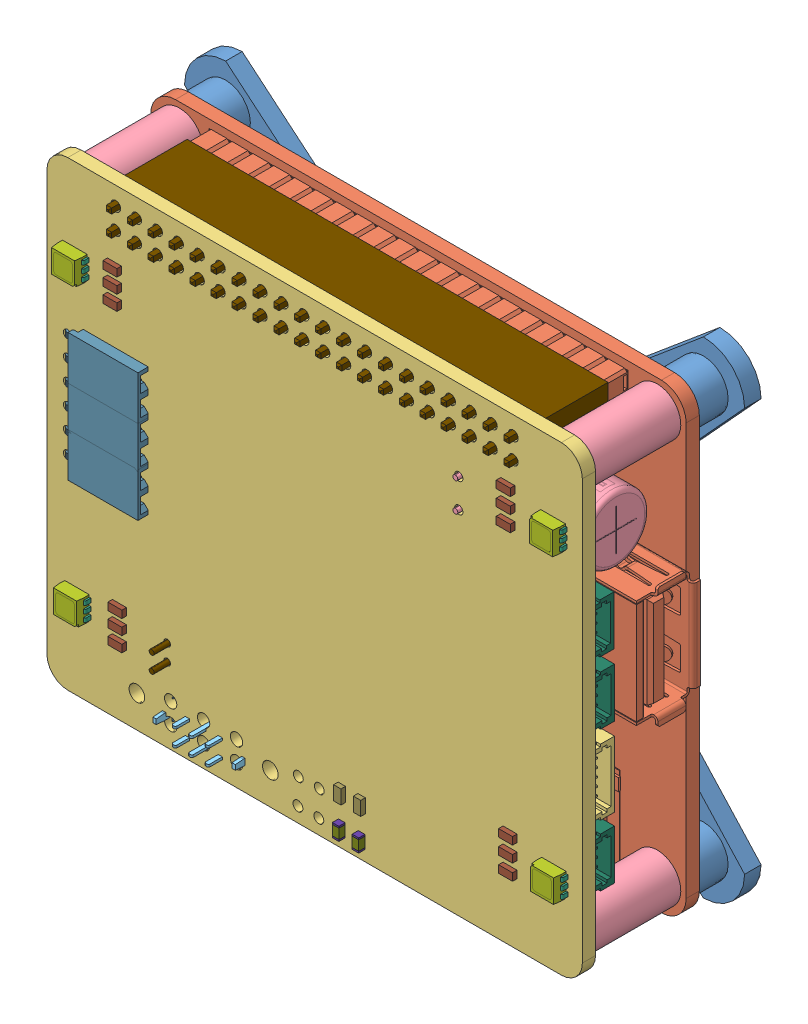
SolidWorks assembly ulemine elektroonika.pi3+, configuration Default. Lengths in mm.
Overall size (68.25 60 22.11).
305 component instances, 41 part files, 9 mates.
Components (placement in the parent):
- Raspberry kinnitus v1.1-1: Raspberry kinnitus v1.1 [Default] at (14.7608 -17.7793 -6.33) x (0 1 0) z (1 0 0) size (59 6 68)
- STMf303 hat + RPi 3A+-1: STMf303 hat + RPi 3A+ [Default] at (-28.0333 0.157 -11.5935) size (68.17 58.5 17.95)
  - Raspberry PI 3 Model A+-1: Raspberry PI 3 Model A+ [Défaut] at (135.3946 10.6154 11.2635) size (68.17 58.5 11.94)
  - FC_PiHat_REV1-1: FC_PiHat_REV1 [Default] at (41.2941 -16.4646 23.8635) x (-1 0 0) z (0 0 -1) size (65 56 12.01)
    - FC_PiHat_REV1.step-1: FC_PiHat_REV1.step [Default] at origin size (65 56 12.01)
      - J7FC_PiHat_REV1.step-1: J7FC_PiHat_REV1.step [Default] at origin size (8 4.95 2.96)
        - SM06B-SRSS-TB.step-1: SM06B-SRSS-TB.step [Default] at (13.3 4.6 -0.3) x (1 0 0) z (0 -1 0) size (8 2.96 4.95)
      - C10FC_PiHat_REV1.step-1: C10FC_PiHat_REV1.step [Default] at origin size (13.96 8.06 10.04)
        - User_Library-Cap_electro_8x11_5x3_5mm_RA.step-1: User_Library-Cap_electro_8x11_5x3_5mm_RA.step [Default] at (13.5254 44.5 4) x (0 1 0) z (0 0 1) size (8.06 13.96 10.04)
      - J11FC_PiHat_REV1.step-1: J11FC_PiHat_REV1.step [Default] at origin size (10 6 9.8)
        - User_Library-EG1940-ND.step-1: User_Library-EG1940-ND.step [Default] at (40.9499 0.2249 0) x (1 0 0) z (0 0 1) size (10 6 9.8)
      - D4FC_PiHat_REV1.step-1: D4FC_PiHat_REV1.step [Default] at origin size (3.4 2.8 1.85)
        - User_Library-RGB_LED_Zwart_ASMT-YTC2-0AA02.step-1: User_Library-RGB_LED_Zwart_ASMT-YTC2-0AA02.step [Default] at (2.2908 8.9737 -1.6023) x (-1 0 0) z (0 -1 0) size (3.4 1.85 2.8)
          - Pootje_RGB_LED.step-1: Pootje_RGB_LED.step [Default] at (-0.3594 -0.1975 0.3238) size (0.9 1.1 0.5)
          - ASMT-YTC2-0AA02.step-1: ASMT-YTC2-0AA02.step [Default] at (-2.6594 -0.3475 0.5738) size (3 1.8 2.8)
          - Pootje_RGB_LED.step-2: Pootje_RGB_LED.step [Default] at (-0.3594 -0.1975 -0.5762) size (0.9 1.1 0.5)
          - Pootje_RGB_LED.step-3: Pootje_RGB_LED.step [Default] at (-0.3594 -0.1975 -1.4762) size (0.9 1.1 0.5)
          - Pootje_RGB_LED.step-4: Pootje_RGB_LED.step [Default] at (-1.9594 -0.1975 -1.9762) x (-1 0 0) z (0 0 -1) size (0.9 1.1 0.5)
          - Pootje_RGB_LED.step-5: Pootje_RGB_LED.step [Default] at (-1.9594 -0.1975 -1.0762) x (-1 0 0) z (0 0 -1) size (0.9 1.1 0.5)
          - Pootje_RGB_LED.step-6: Pootje_RGB_LED.step [Default] at (-1.9594 -0.1975 -0.1762) x (-1 0 0) z (0 0 -1) size (0.9 1.1 0.5)
      - D3FC_PiHat_REV1.step-1: D3FC_PiHat_REV1.step [Default] at origin size (3.4 2.8 1.85)
        - User_Library-RGB_LED_Zwart_ASMT-YTC2-0AA02.step-1: User_Library-RGB_LED_Zwart_ASMT-YTC2-0AA02.step [Default] at (2.3908 45.4737 -1.6023) x (-1 0 0) z (0 -1 0) size (3.4 1.85 2.8)
          - Pootje_RGB_LED.step-1: Pootje_RGB_LED.step [Default] at (-0.3594 -0.1975 0.3238) size (0.9 1.1 0.5)
          - ASMT-YTC2-0AA02.step-1: ASMT-YTC2-0AA02.step [Default] at (-2.6594 -0.3475 0.5738) size (3 1.8 2.8)
          - Pootje_RGB_LED.step-2: Pootje_RGB_LED.step [Default] at (-0.3594 -0.1975 -0.5762) size (0.9 1.1 0.5)
          - Pootje_RGB_LED.step-3: Pootje_RGB_LED.step [Default] at (-0.3594 -0.1975 -1.4762) size (0.9 1.1 0.5)
          - Pootje_RGB_LED.step-4: Pootje_RGB_LED.step [Default] at (-1.9594 -0.1975 -1.9762) x (-1 0 0) z (0 0 -1) size (0.9 1.1 0.5)
          - Pootje_RGB_LED.step-5: Pootje_RGB_LED.step [Default] at (-1.9594 -0.1975 -1.0762) x (-1 0 0) z (0 0 -1) size (0.9 1.1 0.5)
          - Pootje_RGB_LED.step-6: Pootje_RGB_LED.step [Default] at (-1.9594 -0.1975 -0.1762) x (-1 0 0) z (0 0 -1) size (0.9 1.1 0.5)
      - D2FC_PiHat_REV1.step-1: D2FC_PiHat_REV1.step [Default] at origin size (3.4 2.8 1.85)
        - User_Library-RGB_LED_Zwart_ASMT-YTC2-0AA02.step-1: User_Library-RGB_LED_Zwart_ASMT-YTC2-0AA02.step [Default] at (62.5092 10.7763 -1.6023) x (1 0 0) z (0 1 0) size (3.4 1.85 2.8)
          - Pootje_RGB_LED.step-1: Pootje_RGB_LED.step [Default] at (-0.3594 -0.1975 0.3238) size (0.9 1.1 0.5)
          - ASMT-YTC2-0AA02.step-1: ASMT-YTC2-0AA02.step [Default] at (-2.6594 -0.3475 0.5738) size (3 1.8 2.8)
          - Pootje_RGB_LED.step-2: Pootje_RGB_LED.step [Default] at (-0.3594 -0.1975 -0.5762) size (0.9 1.1 0.5)
          - Pootje_RGB_LED.step-3: Pootje_RGB_LED.step [Default] at (-0.3594 -0.1975 -1.4762) size (0.9 1.1 0.5)
          - Pootje_RGB_LED.step-4: Pootje_RGB_LED.step [Default] at (-1.9594 -0.1975 -1.9762) x (-1 0 0) z (0 0 -1) size (0.9 1.1 0.5)
          - Pootje_RGB_LED.step-5: Pootje_RGB_LED.step [Default] at (-1.9594 -0.1975 -1.0762) x (-1 0 0) z (0 0 -1) size (0.9 1.1 0.5)
          - Pootje_RGB_LED.step-6: Pootje_RGB_LED.step [Default] at (-1.9594 -0.1975 -0.1762) x (-1 0 0) z (0 0 -1) size (0.9 1.1 0.5)
      - D1FC_PiHat_REV1.step-1: D1FC_PiHat_REV1.step [Default] at origin size (3.4 2.8 1.85)
        - User_Library-RGB_LED_Zwart_ASMT-YTC2-0AA02.step-1: User_Library-RGB_LED_Zwart_ASMT-YTC2-0AA02.step [Default] at (62.7592 46.4263 -1.6023) x (1 0 0) z (0 1 0) size (3.4 1.85 2.8)
          - Pootje_RGB_LED.step-1: Pootje_RGB_LED.step [Default] at (-0.3594 -0.1975 0.3238) size (0.9 1.1 0.5)
          - ASMT-YTC2-0AA02.step-1: ASMT-YTC2-0AA02.step [Default] at (-2.6594 -0.3475 0.5738) size (3 1.8 2.8)
          - Pootje_RGB_LED.step-2: Pootje_RGB_LED.step [Default] at (-0.3594 -0.1975 -0.5762) size (0.9 1.1 0.5)
          - Pootje_RGB_LED.step-3: Pootje_RGB_LED.step [Default] at (-0.3594 -0.1975 -1.4762) size (0.9 1.1 0.5)
          - Pootje_RGB_LED.step-4: Pootje_RGB_LED.step [Default] at (-1.9594 -0.1975 -1.9762) x (-1 0 0) z (0 0 -1) size (0.9 1.1 0.5)
          - Pootje_RGB_LED.step-5: Pootje_RGB_LED.step [Default] at (-1.9594 -0.1975 -1.0762) x (-1 0 0) z (0 0 -1) size (0.9 1.1 0.5)
          - Pootje_RGB_LED.step-6: Pootje_RGB_LED.step [Default] at (-1.9594 -0.1975 -0.1762) x (-1 0 0) z (0 0 -1) size (0.9 1.1 0.5)
      - S1FC_PiHat_REV1.step-1: S1FC_PiHat_REV1.step [Default] at origin size (4.1 4.1 0.81)
        - 5843174976.step-1: 5843174976.step [Default] at (40.7 32.3 0) size (4.1 4.1 0.81)
          - Body.step-1: Body.step [Default] at (-2.05 -2.05 0)
            - Open_CASCADE_STEP_translator_6.8_14.2.1.x_t-1: Open_CASCADE_STEP_translator_6.8_14.2.1.x_t [Default] at origin
          - Open_CASCADE_STEP_translator_6.8_14.1.step-1: Open_CASCADE_STEP_translator_6.8_14.1.step [Default] at (-2.05 -2.05 0) size (0.52 0.52 0.01)
          - Thermal_Shape.step-1: Thermal_Shape.step [Default] at (-1.3 -1.35 -0.001) size (2.6 2.7 0)
          - Pin_Shape.step-1: Pin_Shape.step [Default] at (-2.05 -1.37 0) size (0.35 0.24 0)
          - Pin_Shape.step-2: Pin_Shape.step [Default] at (2.05 1.37 0) x (-1 0 0) z (0 0 1) size (0.35 0.24 0)
          - Pin_Shape.step-3: Pin_Shape.step [Default] at (-2.05 -0.87 0) size (0.35 0.24 0)
          - Pin_Shape.step-4: Pin_Shape.step [Default] at (2.05 0.87 0) x (-1 0 0) z (0 0 1) size (0.35 0.24 0)
          - Pin_Shape.step-5: Pin_Shape.step [Default] at (-2.05 -0.37 0) size (0.35 0.24 0)
          - Pin_Shape.step-6: Pin_Shape.step [Default] at (2.05 0.37 0) x (-1 0 0) z (0 0 1) size (0.35 0.24 0)
          - Pin_Shape.step-7: Pin_Shape.step [Default] at (-2.05 0.13 0) size (0.35 0.24 0)
          - Pin_Shape.step-8: Pin_Shape.step [Default] at (2.05 -0.13 0) x (-1 0 0) z (0 0 1) size (0.35 0.24 0)
          - Pin_Shape.step-9: Pin_Shape.step [Default] at (-2.05 0.63 0) size (0.35 0.24 0)
          - Pin_Shape.step-10: Pin_Shape.step [Default] at (2.05 -0.63 0) x (-1 0 0) z (0 0 1) size (0.35 0.24 0)
          - Pin_Shape.step-11: Pin_Shape.step [Default] at (-2.05 1.13 0) size (0.35 0.24 0)
          - Pin_Shape.step-12: Pin_Shape.step [Default] at (2.05 -1.13 0) x (-1 0 0) z (0 0 1) size (0.35 0.24 0)
          - Pin_Shape.step-13: Pin_Shape.step [Default] at (-1.13 -2.05 0) x (0 1 0) z (0 0 1) size (0.35 0.24 0)
          - Pin_Shape.step-14: Pin_Shape.step [Default] at (1.13 2.05 0) x (0 -1 0) z (0 0 1) size (0.35 0.24 0)
          - Pin_Shape.step-15: Pin_Shape.step [Default] at (-0.63 -2.05 0) x (0 1 0) z (0 0 1) size (0.35 0.24 0)
          - Pin_Shape.step-16: Pin_Shape.step [Default] at (0.63 2.05 0) x (0 -1 0) z (0 0 1) size (0.35 0.24 0)
          - Pin_Shape.step-17: Pin_Shape.step [Default] at (-0.13 -2.05 0) x (0 1 0) z (0 0 1) size (0.35 0.24 0)
          - Pin_Shape.step-18: Pin_Shape.step [Default] at (0.13 2.05 0) x (0 -1 0) z (0 0 1) size (0.35 0.24 0)
          - Pin_Shape.step-19: Pin_Shape.step [Default] at (0.37 -2.05 0) x (0 1 0) z (0 0 1) size (0.35 0.24 0)
          - Pin_Shape.step-20: Pin_Shape.step [Default] at (-0.37 2.05 0) x (0 -1 0) z (0 0 1) size (0.35 0.24 0)
          - Pin_Shape.step-21: Pin_Shape.step [Default] at (0.87 -2.05 0) x (0 1 0) z (0 0 1) size (0.35 0.24 0)
          - Pin_Shape.step-22: Pin_Shape.step [Default] at (-0.87 2.05 0) x (0 -1 0) z (0 0 1) size (0.35 0.24 0)
          - Pin_Shape.step-23: Pin_Shape.step [Default] at (1.37 -2.05 0) x (0 1 0) z (0 0 1) size (0.35 0.24 0)
          - Pin_Shape.step-24: Pin_Shape.step [Default] at (-1.37 2.05 0) x (0 -1 0) z (0 0 1) size (0.35 0.24 0)
      - R14FC_PiHat_REV1.step-1: R14FC_PiHat_REV1.step [Default] at origin size (1.7 0.9 0.55)
        - 6063442624.step-1: 6063442624.step [Default] at (8.7742 7.9 -2.1523) size (1.7 0.9 0.55)
          - Extruded.step-1: Extruded.step [Default] at origin size (1.7 0.9 0.55)
      - R13FC_PiHat_REV1.step-1: R13FC_PiHat_REV1.step [Default] at origin size (1.7 0.9 0.55)
        - 6063442624.step-1: 6063442624.step [Default] at (8.7742 9.8048 -2.1523) size (1.7 0.9 0.55)
          - Extruded.step-1: Extruded.step [Default] at origin size (1.7 0.9 0.55)
      - R12FC_PiHat_REV1.step-1: R12FC_PiHat_REV1.step [Default] at origin size (1.7 0.9 0.55)
        - 6063442624.step-1: 6063442624.step [Default] at (8.7742 11.7 -2.1523) size (1.7 0.9 0.55)
          - Extruded.step-1: Extruded.step [Default] at origin size (1.7 0.9 0.55)
      - R11FC_PiHat_REV1.step-1: R11FC_PiHat_REV1.step [Default] at origin size (1.7 0.9 0.55)
        - 6063442624.step-1: 6063442624.step [Default] at (9.05 44.4 -2.1523) size (1.7 0.9 0.55)
          - Extruded.step-1: Extruded.step [Default] at origin size (1.7 0.9 0.55)
      - R10FC_PiHat_REV1.step-1: R10FC_PiHat_REV1.step [Default] at origin size (1.7 0.9 0.55)
        - 6063442624.step-1: 6063442624.step [Default] at (9.05 46.3 -2.1523) size (1.7 0.9 0.55)
          - Extruded.step-1: Extruded.step [Default] at origin size (1.7 0.9 0.55)
      - R9FC_PiHat_REV1.step-1: R9FC_PiHat_REV1.step [Default] at origin size (0.9 1.7 0.55)
        - 6063442432.step-1: 6063442432.step [Default] at (59.9 29.7 0) size (0.9 1.7 0.55)
          - Extruded-0.step-1: Extruded-0.step [Default] at origin size (0.9 1.7 0.55)
      - R8FC_PiHat_REV1.step-1: R8FC_PiHat_REV1.step [Default] at origin size (1.7 0.9 0.55)
        - 6063442624.step-1: 6063442624.step [Default] at (9.05 48.2 -2.1523) size (1.7 0.9 0.55)
          - Extruded.step-1: Extruded.step [Default] at origin size (1.7 0.9 0.55)
      - R7FC_PiHat_REV1.step-1: R7FC_PiHat_REV1.step [Default] at origin size (1.84 1.84 0.55)
        - 6063441088.step-1: 6063441088.step [Default] at (39.9 37.9 0) size (1.84 1.84 0.55)
          - Extruded-1.step-1: Extruded-1.step [Default] at origin size (1.84 1.84 0.55)
      - R6FC_PiHat_REV1.step-1: R6FC_PiHat_REV1.step [Default] at origin size (1.7 0.9 0.55)
        - 6063442624.step-1: 6063442624.step [Default] at (56.2 11.8 -2.1523) size (1.7 0.9 0.55)
          - Extruded.step-1: Extruded.step [Default] at origin size (1.7 0.9 0.55)
      - R5FC_PiHat_REV1.step-1: R5FC_PiHat_REV1.step [Default] at origin size (1.7 0.9 0.55)
        - 6063442624.step-1: 6063442624.step [Default] at (56.2 10 -2.1523) size (1.7 0.9 0.55)
          - Extruded.step-1: Extruded.step [Default] at origin size (1.7 0.9 0.55)
      - R4FC_PiHat_REV1.step-1: R4FC_PiHat_REV1.step [Default] at origin size (1.7 0.9 0.55)
        - 6063442624.step-1: 6063442624.step [Default] at (56.2 8.2 -2.1523) size (1.7 0.9 0.55)
          - Extruded.step-1: Extruded.step [Default] at origin size (1.7 0.9 0.55)
      - R3FC_PiHat_REV1.step-1: R3FC_PiHat_REV1.step [Default] at origin size (1.7 0.9 0.55)
        - 6063442624.step-1: 6063442624.step [Default] at (56.8 47.4 -2.1523) size (1.7 0.9 0.55)
          - Extruded.step-1: Extruded.step [Default] at origin size (1.7 0.9 0.55)
      - R2FC_PiHat_REV1.step-1: R2FC_PiHat_REV1.step [Default] at origin size (1.7 0.9 0.55)
        - 6063442624.step-1: 6063442624.step [Default] at (56.8 45.6 -2.1523) size (1.7 0.9 0.55)
          - Extruded.step-1: Extruded.step [Default] at origin size (1.7 0.9 0.55)
      - R1FC_PiHat_REV1.step-1: R1FC_PiHat_REV1.step [Default] at origin size (1.7 0.9 0.55)
        - 6063442624.step-1: 6063442624.step [Default] at (56.8 43.8 -2.1523) size (1.7 0.9 0.55)
          - Extruded.step-1: Extruded.step [Default] at origin size (1.7 0.9 0.55)
      - J8FC_PiHat_REV1.step-1: J8FC_PiHat_REV1.step [Default] at origin size (4.95 8 2.96)
        - SM06B-SRSS-TB.step-1: SM06B-SRSS-TB.step [Default] at (4.55 19.8 -0.3) x (0 -1 0) z (-1 0 0) size (8 2.96 4.95)
      - J6FC_PiHat_REV1.step-1: J6FC_PiHat_REV1.step [Default] at origin size (10.06 15.53 5.7)
        - female_header_a-bl254-ea-g02d.step-1: female_header_a-bl254-ea-g02d.step [Default] at (61.2001 31.0851 -1.6023) x (0 -1 0) z (0 0 -1) size (5.33 10.06 5.7)
        - female_header_a-bl254-ea-g02d.step-2: female_header_a-bl254-ea-g02d.step [Default] at (61.2001 26.0099 -1.6023) x (0 -1 0) z (0 0 -1) size (5.33 10.06 5.7)
        - female_header_a-bl254-ea-g02d.step-3: female_header_a-bl254-ea-g02d.step [Default] at (61.2001 36.2099 -1.6023) x (0 -1 0) z (0 0 -1) size (5.33 10.06 5.7)
      - J4FC_PiHat_REV1.step-1: J4FC_PiHat_REV1.step [Default] at origin size (4.95 6 2.96)
        - SM04B-SRSS-TB.step-1: SM04B-SRSS-TB.step [Default] at (4.55 28.375 -0.3) x (0 -1 0) z (-1 0 0) size (6 2.96 4.95)
      - J3FC_PiHat_REV1.step-1: J3FC_PiHat_REV1.step [Default] at origin size (4.95 6 2.96)
        - SM04B-SRSS-TB.step-1: SM04B-SRSS-TB.step [Default] at (4.55 11.35 -0.3) x (0 -1 0) z (-1 0 0) size (6 2.96 4.95)
      - J2FC_PiHat_REV1.step-1: J2FC_PiHat_REV1.step [Default] at origin size (8 4.95 2.96)
        - SM06B-SRSS-TB.step-1: SM06B-SRSS-TB.step [Default] at (22.8093 4.575 -0.3) x (1 0 0) z (0 -1 0) size (8 2.96 4.95)
      - J1FC_PiHat_REV1.step-1: J1FC_PiHat_REV1.step [Default] at origin size (4.95 6 2.96)
        - SM04B-SRSS-TB.step-1: SM04B-SRSS-TB.step [Default] at (4.625 35.925 -0.3) x (0 -1 0) z (-1 0 0) size (6 2.96 4.95)
      - C4FC_PiHat_REV1.step-1: C4FC_PiHat_REV1.step [Default] at origin size (0.9 1.8 0.9)
        - 6063440896.step-1: 6063440896.step [Default] at (41.3 27.825 0) size (0.9 1.8 0.9)
          - Extruded-2.step-1: Extruded-2.step [Default] at origin size (0.9 1.8 0.9)
      - C3FC_PiHat_REV1.step-1: C3FC_PiHat_REV1.step [Default] at origin size (0.9 1.8 0.9)
        - 6063440896.step-1: 6063440896.step [Default] at (44.1 32.225 0) size (0.9 1.8 0.9)
          - Extruded-2.step-1: Extruded-2.step [Default] at origin size (0.9 1.8 0.9)
      - C2FC_PiHat_REV1.step-1: C2FC_PiHat_REV1.step [Default] at origin size (1.8 0.9 0.9)
        - 6063441280.step-1: 6063441280.step [Default] at (38.125 28.8 0) size (1.8 0.9 0.9)
          - Extruded-3.step-1: Extruded-3.step [Default] at origin size (1.8 0.9 0.9)
      - C1FC_PiHat_REV1.step-1: C1FC_PiHat_REV1.step [Default] at origin size (1.8 0.9 0.9)
        - 6063441280.step-1: 6063441280.step [Default] at (38.125 26.7 0) size (1.8 0.9 0.9)
          - Extruded-3.step-1: Extruded-3.step [Default] at origin size (1.8 0.9 0.9)
      - J5FC_PiHat_REV1.step-1: J5FC_PiHat_REV1.step [Default] at origin size (51.1 5 11.1)
        - User_Library-Header_2x20_2_54mm.step-1: User_Library-Header_2x20_2_54mm.step [Default] at (56.6601 52.5601 0) x (1 0 0) z (0 -1 0) size (51.1 11.1 5)
      - L2FC_PiHat_REV1.step-1: L2FC_PiHat_REV1.step [Default] at origin size (12.5 12.7 6.1)
        - 5843174592.step-1: 5843174592.step [Default] at (40.7 17.6 0) x (0 1 0) z (0 0 1) size (12.7 12.5 6.1)
          - pin.step-1: pin.step [Default] at (6.35 2.8 0) x (-1 0 0) z (0 0 1) size (4.5 5.6 3)
            - Open_CASCADE_STEP_translator_6.8_3.3.1.step-1: Open_CASCADE_STEP_translator_6.8_3.3.1.step [Default] at origin size (4.5 5.6 3)
          - pin.step-2: pin.step [Default] at (-6.35 -2.8 0) size (4.5 5.6 3)
            - Open_CASCADE_STEP_translator_6.8_3.3.1.step-1: Open_CASCADE_STEP_translator_6.8_3.3.1.step [Default] at origin size (4.5 5.6 3)
          - Body.step-1: Body.step [Default] at (0 0 0.1)
            - Open_CASCADE_STEP_translator_6.8_14.2.1.x_t-1: Open_CASCADE_STEP_translator_6.8_14.2.1.x_t [Default] at origin
          - cylinder.step-1: cylinder.step [Default] at (0 0 0.1) size (12.5 12.5 3)
      - U3FC_PiHat_REV1.step-1: U3FC_PiHat_REV1.step [Default] at origin size (10.3 15.24 4.47)
        - 5843175168.step-1: 5843175168.step [Default] at (52.775 32.425 0) x (0 1 0) z (0 0 1) size (15.24 10.3 4.47)
          - Body-1.step-1: Body-1.step [Default] at (-4.575 -5.15 0) size (9.15 10.3 4.47)
            - Open_CASCADE_STEP_translator_6.8_42.2.1.step-1: Open_CASCADE_STEP_translator_6.8_42.2.1.step [Default] at origin size (9.15 10.3 4.47)
          - tab.step-1: tab.step [Default] at (-4.575 -5.15 0) size (9 10.25 0.35)
            - Open_CASCADE_STEP_translator_6.8_42.8.1.step-1: Open_CASCADE_STEP_translator_6.8_42.8.1.step [Default] at origin size (9 10.25 0.35)
          - Open_CASCADE_STEP_translator_6.8_42.1.step-1: Open_CASCADE_STEP_translator_6.8_42.1.step [Default] at (-4.575 -5.15 0) size (1.3 1.3 0.01)
          - Lead.step-1: Lead.step [Default] at (-4.575 -3.4 0) x (-1 0 0) z (0 0 1) size (5.46 0.75 2.33)
          - Lead.step-2: Lead.step [Default] at (-4.575 -1.7 0) x (-1 0 0) z (0 0 1) size (5.46 0.75 2.33)
          - Lead.step-3: Lead.step [Default] at (-4.575 0 0) x (-1 0 0) z (0 0 1) size (5.46 0.75 2.33)
          - Lead.step-4: Lead.step [Default] at (-4.575 1.7 0) x (-1 0 0) z (0 0 1) size (5.46 0.75 2.33)
          - Lead.step-5: Lead.step [Default] at (-4.575 3.4 0) x (-1 0 0) z (0 0 1) size (5.46 0.75 2.33)
        - 5843175168-4.step-1: 5843175168-4.step [Default] at (52.775 32.425 0) x (0 1 0) z (0 0 1) size (2.73 0.75 0.2)
      - D6FC_PiHat_REV1.step-1: D6FC_PiHat_REV1.step [Default] at origin size (7.55 6.23 2.62)
        - 5843175552.step-1: 5843175552.step [Default] at (51.8001 16.8001 0) x (1 0 0) z (0 0 1) size (7.55 6.22 2.62)
          - Body-2.step-1: Body-2.step [Default] at (-3.555 -3.11 0.25) size (7.12 6.22 2.47)
            - Open_CASCADE_STEP_translator_6.8_45.1.1.step-1: Open_CASCADE_STEP_translator_6.8_45.1.1.step [Default] at origin size (7.12 6.22 2.47)
          - Lead-5.step-1: Lead-5.step [Default] at (2.635 0 0) size (1.14 3 1.53)
          - Lead-5.step-2: Lead-5.step [Default] at (-2.635 0 0) x (-1 0 0) z (0 0 1) size (1.14 3 1.53)
      - U2FC_PiHat_REV1.step-1: U2FC_PiHat_REV1.step [Default] at origin size (3.98 3.97 1)
        - 5843176128.step-1: 5843176128.step [Default] at (49.3313 45.4354 0) x (0.707107 -0.707107 0) z (0 0 1) size (2.8 2.91 1)
          - Body-3.step-1: Body-3.step [Default] at (-0.8 -1.45 0) size (1.6 2.91 0.95)
            - Open_CASCADE_STEP_translator_6.8_3.1.1.step-1: Open_CASCADE_STEP_translator_6.8_3.1.1.step [Default] at origin size (1.6 2.91 0.95)
          - Leader.step-1: Leader.step [Default] at (-0.8 -0.95 0) x (-1 0 0) z (0 0 1) size (0.6 0.5 0.57)
          - Leader.step-2: Leader.step [Default] at (-0.8 0 0) x (-1 0 0) z (0 0 1) size (0.6 0.5 0.57)
          - Leader.step-3: Leader.step [Default] at (-0.8 0.95 0) x (-1 0 0) z (0 0 1) size (0.6 0.5 0.57)
          - Leader.step-4: Leader.step [Default] at (0.8 -0.95 0) size (0.6 0.5 0.57)
          - Leader.step-5: Leader.step [Default] at (0.8 0.95 0) size (0.6 0.5 0.57)
      - U1FC_PiHat_REV1.step-1: U1FC_PiHat_REV1.step [Default] at origin size (18.98 19.05 1.5)
        - 5843174208.step-1: 5843174208.step [Default] at (26.375 36.65 0) x (-0.707107 -0.707107 0) z (0 0 1) size (14.7 14.7 1.5)
          - Body-4.step-1: Body-4.step [Default] at (-5 -5 0) size (10 10 1.5)
            - Open_CASCADE_STEP_translator_6.8_6.1.1.step-1: Open_CASCADE_STEP_translator_6.8_6.1.1.step [Default] at origin size (10 10 1.5)
          - Leader-6.step-1: Leader-6.step [Default] at (-5 -3.75 0) x (-1 0 0) z (0 0 1) size (2.35 0.27 0.85)
          - Leader-6.step-2: Leader-6.step [Default] at (-3.75 5 0) x (0 1 0) z (0 0 1) size (2.35 0.27 0.85)
          - Leader-6.step-3: Leader-6.step [Default] at (5 -3.75 0) size (2.35 0.27 0.85)
          - Leader-6.step-4: Leader-6.step [Default] at (-3.75 -5 0) x (0 -1 0) z (0 0 1) size (2.35 0.27 0.85)
          - Leader-6.step-5: Leader-6.step [Default] at (-5 -3.25 0) x (-1 0 0) z (0 0 1) size (2.35 0.27 0.85)
          - Leader-6.step-6: Leader-6.step [Default] at (-3.25 5 0) x (0 1 0) z (0 0 1) size (2.35 0.27 0.85)
          - Leader-6.step-7: Leader-6.step [Default] at (5 -3.25 0) size (2.35 0.27 0.85)
          - Leader-6.step-8: Leader-6.step [Default] at (-3.25 -5 0) x (0 -1 0) z (0 0 1) size (2.35 0.27 0.85)
          - Leader-6.step-9: Leader-6.step [Default] at (-5 -2.75 0) x (-1 0 0) z (0 0 1) size (2.35 0.27 0.85)
          - Leader-6.step-10: Leader-6.step [Default] at (-2.75 5 0) x (0 1 0) z (0 0 1) size (2.35 0.27 0.85)
          - Leader-6.step-11: Leader-6.step [Default] at (5 -2.75 0) size (2.35 0.27 0.85)
          - Leader-6.step-12: Leader-6.step [Default] at (-2.75 -5 0) x (0 -1 0) z (0 0 1) size (2.35 0.27 0.85)
          - Leader-6.step-13: Leader-6.step [Default] at (-5 -2.25 0) x (-1 0 0) z (0 0 1) size (2.35 0.27 0.85)
          - Leader-6.step-14: Leader-6.step [Default] at (-2.25 5 0) x (0 1 0) z (0 0 1) size (2.35 0.27 0.85)
          - Leader-6.step-15: Leader-6.step [Default] at (5 -2.25 0) size (2.35 0.27 0.85)
          - Leader-6.step-16: Leader-6.step [Default] at (-2.25 -5 0) x (0 -1 0) z (0 0 1) size (2.35 0.27 0.85)
          - Leader-6.step-17: Leader-6.step [Default] at (-5 -1.75 0) x (-1 0 0) z (0 0 1) size (2.35 0.27 0.85)
          - Leader-6.step-18: Leader-6.step [Default] at (-1.75 5 0) x (0 1 0) z (0 0 1) size (2.35 0.27 0.85)
          - Leader-6.step-19: Leader-6.step [Default] at (5 -1.75 0) size (2.35 0.27 0.85)
          - Leader-6.step-20: Leader-6.step [Default] at (-1.75 -5 0) x (0 -1 0) z (0 0 1) size (2.35 0.27 0.85)
          - Leader-6.step-21: Leader-6.step [Default] at (-5 -1.25 0) x (-1 0 0) z (0 0 1) size (2.35 0.27 0.85)
          - Leader-6.step-22: Leader-6.step [Default] at (-1.25 5 0) x (0 1 0) z (0 0 1) size (2.35 0.27 0.85)
          - Leader-6.step-23: Leader-6.step [Default] at (5 -1.25 0) size (2.35 0.27 0.85)
          - Leader-6.step-24: Leader-6.step [Default] at (-1.25 -5 0) x (0 -1 0) z (0 0 1) size (2.35 0.27 0.85)
          - Leader-6.step-25: Leader-6.step [Default] at (-5 -0.75 0) x (-1 0 0) z (0 0 1) size (2.35 0.27 0.85)
          - Leader-6.step-26: Leader-6.step [Default] at (-0.75 5 0) x (0 1 0) z (0 0 1) size (2.35 0.27 0.85)
          - Leader-6.step-27: Leader-6.step [Default] at (5 -0.75 0) size (2.35 0.27 0.85)
          - Leader-6.step-28: Leader-6.step [Default] at (-0.75 -5 0) x (0 -1 0) z (0 0 1) size (2.35 0.27 0.85)
          - Leader-6.step-29: Leader-6.step [Default] at (-5 -0.25 0) x (-1 0 0) z (0 0 1) size (2.35 0.27 0.85)
          - Leader-6.step-30: Leader-6.step [Default] at (-0.25 5 0) x (0 1 0) z (0 0 1) size (2.35 0.27 0.85)
          - Leader-6.step-31: Leader-6.step [Default] at (5 -0.25 0) size (2.35 0.27 0.85)
          - Leader-6.step-32: Leader-6.step [Default] at (-0.25 -5 0) x (0 -1 0) z (0 0 1) size (2.35 0.27 0.85)
          - Leader-6.step-33: Leader-6.step [Default] at (-5 0.25 0) x (-1 0 0) z (0 0 1) size (2.35 0.27 0.85)
          - Leader-6.step-34: Leader-6.step [Default] at (0.25 5 0) x (0 1 0) z (0 0 1) size (2.35 0.27 0.85)
          - Leader-6.step-35: Leader-6.step [Default] at (5 0.25 0) size (2.35 0.27 0.85)
          - Leader-6.step-36: Leader-6.step [Default] at (0.25 -5 0) x (0 -1 0) z (0 0 1) size (2.35 0.27 0.85)
          - Leader-6.step-37: Leader-6.step [Default] at (-5 0.75 0) x (-1 0 0) z (0 0 1) size (2.35 0.27 0.85)
          - Leader-6.step-38: Leader-6.step [Default] at (0.75 5 0) x (0 1 0) z (0 0 1) size (2.35 0.27 0.85)
          - Leader-6.step-39: Leader-6.step [Default] at (5 0.75 0) size (2.35 0.27 0.85)
          - Leader-6.step-40: Leader-6.step [Default] at (0.75 -5 0) x (0 -1 0) z (0 0 1) size (2.35 0.27 0.85)
          - Leader-6.step-41: Leader-6.step [Default] at (-5 1.25 0) x (-1 0 0) z (0 0 1) size (2.35 0.27 0.85)
          - Leader-6.step-42: Leader-6.step [Default] at (1.25 5 0) x (0 1 0) z (0 0 1) size (2.35 0.27 0.85)
          - Leader-6.step-43: Leader-6.step [Default] at (5 1.25 0) size (2.35 0.27 0.85)
          - Leader-6.step-44: Leader-6.step [Default] at (1.25 -5 0) x (0 -1 0) z (0 0 1) size (2.35 0.27 0.85)
          - Leader-6.step-45: Leader-6.step [Default] at (-5 1.75 0) x (-1 0 0) z (0 0 1) size (2.35 0.27 0.85)
          - Leader-6.step-46: Leader-6.step [Default] at (1.75 5 0) x (0 1 0) z (0 0 1) size (2.35 0.27 0.85)
          - Leader-6.step-47: Leader-6.step [Default] at (5 1.75 0) size (2.35 0.27 0.85)
          - Leader-6.step-48: Leader-6.step [Default] at (1.75 -5 0) x (0 -1 0) z (0 0 1) size (2.35 0.27 0.85)
          - Leader-6.step-49: Leader-6.step [Default] at (-5 2.25 0) x (-1 0 0) z (0 0 1) size (2.35 0.27 0.85)
          - Leader-6.step-50: Leader-6.step [Default] at (2.25 5 0) x (0 1 0) z (0 0 1) size (2.35 0.27 0.85)
          - Leader-6.step-51: Leader-6.step [Default] at (5 2.25 0) size (2.35 0.27 0.85)
          - Leader-6.step-52: Leader-6.step [Default] at (2.25 -5 0) x (0 -1 0) z (0 0 1) size (2.35 0.27 0.85)
          - Leader-6.step-53: Leader-6.step [Default] at (-5 2.75 0) x (-1 0 0) z (0 0 1) size (2.35 0.27 0.85)
          - Leader-6.step-54: Leader-6.step [Default] at (2.75 5 0) x (0 1 0) z (0 0 1) size (2.35 0.27 0.85)
          - Leader-6.step-55: Leader-6.step [Default] at (5 2.75 0) size (2.35 0.27 0.85)
          - Leader-6.step-56: Leader-6.step [Default] at (2.75 -5 0) x (0 -1 0) z (0 0 1) size (2.35 0.27 0.85)
          - Leader-6.step-57: Leader-6.step [Default] at (-5 3.25 0) x (-1 0 0) z (0 0 1) size (2.35 0.27 0.85)
          - Leader-6.step-58: Leader-6.step [Default] at (3.25 5 0) x (0 1 0) z (0 0 1) size (2.35 0.27 0.85)
          - Leader-6.step-59: Leader-6.step [Default] at (5 3.25 0) size (2.35 0.27 0.85)
          - Leader-6.step-60: Leader-6.step [Default] at (3.25 -5 0) x (0 -1 0) z (0 0 1) size (2.35 0.27 0.85)
          - Leader-6.step-61: Leader-6.step [Default] at (-5 3.75 0) x (-1 0 0) z (0 0 1) size (2.35 0.27 0.85)
          - Leader-6.step-62: Leader-6.step [Default] at (3.75 5 0) x (0 1 0) z (0 0 1) size (2.35 0.27 0.85)
          - Leader-6.step-63: Leader-6.step [Default] at (5 3.75 0) size (2.35 0.27 0.85)
          - Leader-6.step-64: Leader-6.step [Default] at (3.75 -5 0) x (0 -1 0) z (0 0 1) size (2.35 0.27 0.85)
      - R17FC_PiHat_REV1.step-1: R17FC_PiHat_REV1.step [Default] at origin size (0.9 1.7 0.55)
        - 6063442432.step-1: 6063442432.step [Default] at (29.2 5.9 -2.1523) size (0.9 1.7 0.55)
          - Extruded-0.step-1: Extruded-0.step [Default] at origin size (0.9 1.7 0.55)
      - R15FC_PiHat_REV1.step-1: R15FC_PiHat_REV1.step [Default] at origin size (0.9 1.7 0.55)
        - 6063442432.step-1: 6063442432.step [Default] at (26.8 5.9 -2.1523) size (0.9 1.7 0.55)
          - Extruded-0.step-1: Extruded-0.step [Default] at origin size (0.9 1.7 0.55)
      - Q1FC_PiHat_REV1.step-1: Q1FC_PiHat_REV1.step [Default] at origin size (3.2 5 1.35)
        - User_Library-445-CRYTAL-SMD.step-1: User_Library-445-CRYTAL-SMD.step [Default] at (37.4671 49.9363 0.0126) x (0 1 0) z (1 0 0) size (5 1.35 3.2)
      - L3FC_PiHat_REV1.step-1: L3FC_PiHat_REV1.step [Default] at origin size (12.5 12.7 6.1)
        - 5843174592.step-1: 5843174592.step [Default] at (27.5 17.6 0) x (0 1 0) z (0 0 1) size (12.7 12.5 6.1)
          - pin.step-1: pin.step [Default] at (6.35 2.8 0) x (-1 0 0) z (0 0 1) size (4.5 5.6 3)
            - Open_CASCADE_STEP_translator_6.8_3.3.1.step-1: Open_CASCADE_STEP_translator_6.8_3.3.1.step [Default] at origin size (4.5 5.6 3)
          - pin.step-2: pin.step [Default] at (-6.35 -2.8 0) size (4.5 5.6 3)
            - Open_CASCADE_STEP_translator_6.8_3.3.1.step-1: Open_CASCADE_STEP_translator_6.8_3.3.1.step [Default] at origin size (4.5 5.6 3)
          - Body.step-1: Body.step [Default] at (0 0 0.1)
            - Open_CASCADE_STEP_translator_6.8_14.2.1.x_t-1: Open_CASCADE_STEP_translator_6.8_14.2.1.x_t [Default] at origin
          - cylinder.step-1: cylinder.step [Default] at (0 0 0.1) size (12.5 12.5 3)
      - L1FC_PiHat_REV1.step-1: L1FC_PiHat_REV1.step [Default] at origin size (3.68 3.68 1.5)
        - 6063441856.step-1: 6063441856.step [Default] at (51.5 42 0) size (3.68 3.68 1.5)
          - Extruded-7.step-1: Extruded-7.step [Default] at origin size (3.68 3.68 1.5)
      - D7FC_PiHat_REV1.step-1: D7FC_PiHat_REV1.step [Default] at origin size (0.8 1.6 0.75)
        - 6063441664.step-1: 6063441664.step [Default] at (29.2 2.1 -2.3523) size (0.8 1.2 0.75)
          - Extruded-8.step-1: Extruded-8.step [Default] at origin size (0.8 1.2 0.75)
        - 6063441472.step-1: 6063441472.step [Default] at (29.2 2.8 -2.3523) size (0.8 0.2 0.75)
          - Extruded-9.step-1: Extruded-9.step [Default] at origin size (0.8 0.2 0.75)
        - 6063441472.step-2: 6063441472.step [Default] at (29.2 1.4 -2.3523) size (0.8 0.2 0.75)
          - Extruded-9.step-1: Extruded-9.step [Default] at origin size (0.8 0.2 0.75)
      - D5FC_PiHat_REV1.step-1: D5FC_PiHat_REV1.step [Default] at origin size (0.8 1.6 0.75)
        - 6063441664.step-1: 6063441664.step [Default] at (26.8 2.075 -2.3523) size (0.8 1.2 0.75)
          - Extruded-8.step-1: Extruded-8.step [Default] at origin size (0.8 1.2 0.75)
        - 6063441472.step-1: 6063441472.step [Default] at (26.8 2.775 -2.3523) size (0.8 0.2 0.75)
          - Extruded-9.step-1: Extruded-9.step [Default] at origin size (0.8 0.2 0.75)
        - 6063441472.step-2: 6063441472.step [Default] at (26.8 1.375 -2.3523) size (0.8 0.2 0.75)
          - Extruded-9.step-1: Extruded-9.step [Default] at origin size (0.8 0.2 0.75)
      - C9FC_PiHat_REV1.step-1: C9FC_PiHat_REV1.step [Default] at origin size (13.46 5.06 8.54)
        - User_Library-Cap_electro_5x11x2mm_RA.step-1: User_Library-Cap_electro_5x11x2mm_RA.step [Default] at (51.885 9.9755 2.5) x (0 -1 0) z (0 0 1) size (5.06 13.46 8.54)
      - C8FC_PiHat_REV1.step-1: C8FC_PiHat_REV1.step [Default] at origin size (1.91 1.91 0.9)
        - 6063442048.step-1: 6063442048.step [Default] at (47.1 43.3857 0) size (1.91 1.91 0.9)
          - Extruded-10.step-1: Extruded-10.step [Default] at origin size (1.91 1.91 0.9)
      - C7FC_PiHat_REV1.step-1: C7FC_PiHat_REV1.step [Default] at origin size (1.91 1.91 0.9)
        - 6063442240.step-1: 6063442240.step [Default] at (45.7 46.4 0) size (1.91 1.91 0.9)
          - Extruded-11.step-1: Extruded-11.step [Default] at origin size (1.91 1.91 0.9)
      - C6FC_PiHat_REV1.step-1: C6FC_PiHat_REV1.step [Default] at origin size (1.8 0.9 0.9)
        - 6063441280.step-1: 6063441280.step [Default] at (39.9535 42.2416 0) size (1.8 0.9 0.9)
          - Extruded-3.step-1: Extruded-3.step [Default] at origin size (1.8 0.9 0.9)
      - C5FC_PiHat_REV1.step-1: C5FC_PiHat_REV1.step [Default] at origin size (1.8 0.9 0.9)
        - 6063441280.step-1: 6063441280.step [Default] at (39.9535 44.9915 0) size (1.8 0.9 0.9)
          - Extruded-3.step-1: Extruded-3.step [Default] at origin size (1.8 0.9 0.9)
      - BoardFC_PiHat_REV1.step-1: BoardFC_PiHat_REV1.step [Default] at origin size (65 56 1.6)
  - Spacer-1: Spacer [Default] at (37.7941 -12.9363 12.8635) x (-1 0 0) z (0 1 0) size (5.7 11 5.7)
  - Spacer-2: Spacer [Default] at (-20.2059 -12.9363 12.8635) x (1 0 0) z (0 -1 0) size (5.7 11 5.7)
  - Spacer-3: Spacer [Default] at (-20.2059 36.0637 12.8635) x (1 0 0) z (0 -1 0) size (5.7 11 5.7)
  - Spacer-4: Spacer [Default] at (37.7941 36.0637 12.8635) x (-1 0 0) z (0 1 0) size (5.7 11 5.7)
Mates (geometry in assembly coordinates):
- Concentric1: concentric anti-aligned: cylinder of Raspberry pi 3 cad model-1/raspberrypi_3_stripped.step-1/Raspberry Pi 31.step-1 through (13.058 26.9107 -0.75) axis (0 0 1) radius 1.375; cylinder of Raspberry kinnitus v1.1-1 through (13.058 26.9107 -4.33) axis (0 0 -1) radius 1
- Concentric2: concentric anti-aligned: cylinder of Raspberry pi 3 cad model-1/raspberrypi_3_stripped.step-1/Raspberry Pi 31.step-1 through (13.058 -22.0893 -0.75) axis (0 0 1) radius 1.375; cylinder of Raspberry kinnitus v1.1-1 through (13.058 -22.0893 -4.33) axis (0 0 -1) radius 1
- Coincident1: coincident anti-aligned: plane of Raspberry pi 3 cad model-1/raspberrypi_3_stripped.step-1/Raspberry Pi 31.step-1 through (36.4822 30.4107 -0.33) normal (0 0 -1); plane of Raspberry kinnitus v1.1-1 through (13.058 26.9107 -0.33) normal (0 0 1)
- Concentric5: concentric anti-aligned: cylinder of Raspberry pi 3 cad model-1/raspberrypi_3_stripped.step-1/Raspberry Pi 31.step-1 through (-44.942 26.9107 -0.75) axis (0 0 1) radius 1.375; cylinder of rasberry kate-1 through (-44.942 26.9107 18.6) axis (0 0 -1) radius 1.375
- Concentric6: concentric aligned: cylinder of Raspberry kinnitus v1.1-1 through (13.058 26.9107 -0.33) axis (0 0 -1) radius 3; cylinder of rasberry kate-1 through (13.058 26.9107 18.6) axis (0 0 -1) radius 1.375
- Coincident3: coincident anti-aligned: plane of Raspberry pi 3 cad model-1/raspberrypi_3_stripped.step-1/Raspberry Pi 31.step-1 through (-48.452 -25.5993 1) normal (0 0 1); plane of rasberry kate-1 through (-44.942 26.9107 1) normal (0 0 -1)
- Concentric7: concentric aligned: cylinder of Raspberry kinnitus v1.1-1 through (-48.2392 36.2207 -4.33) axis (0 0 -1) radius 1; cylinder of STMf303 hat + RPi 3A+-1/Raspberry PI 3 Model A+-1 through (-48.2392 36.2207 1.27) axis (0 0 -1) radius 1.375
- Concentric8: concentric aligned: cylinder of Raspberry kinnitus v1.1-1 through (9.7608 -12.7793 -4.33) axis (0 0 -1) radius 1; cylinder of STMf303 hat + RPi 3A+-1/Raspberry PI 3 Model A+-1 through (9.7608 -12.7793 1.27) axis (0 0 -1) radius 1.375
- Coincident4: coincident anti-aligned: plane of Raspberry kinnitus v1.1-1 through (9.7608 -12.7793 -0.33) normal (0 0 1); plane of STMf303 hat + RPi 3A+-1/Raspberry PI 3 Model A+-1 through (-9.2392 11.7207 -0.33) normal (0 0 -1)
